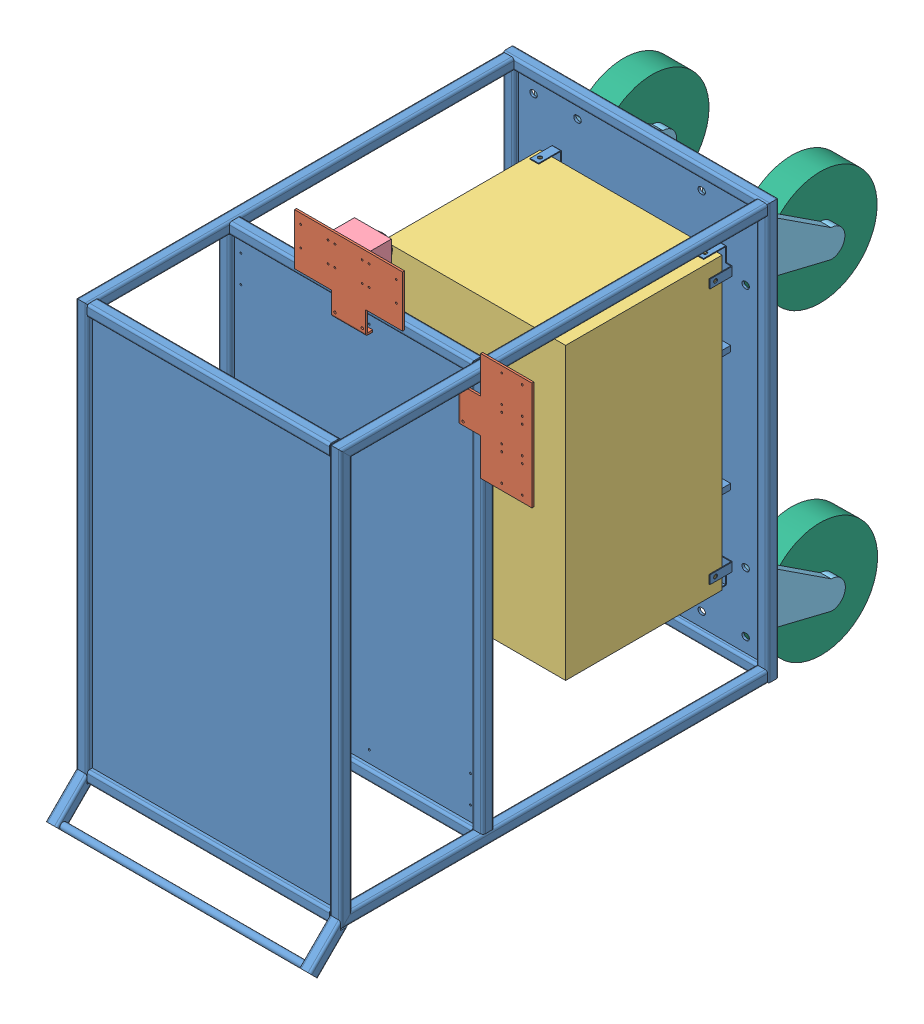
SolidWorks assembly kart, configuration Default. Lengths in mm.
Overall size (555.49 886.14 1699.31).
17 component instances, 6 part files, 21 mates.
Components (placement in the parent):
- kart_skeleton-1: kart_skeleton [Default<A macchina>] at (18.5226 -16.0189 875.6692) size (465.49 783.64 823.64)
- lidar_plate_T-1: lidar_plate_T [Default] at (296.2677 278.9811 1389.6647) x (-1 0 0) z (0 0 1) size (130.26 190 13)
- lidar_plate_T-2: lidar_plate_T [Default] at (18.5226 383.9811 1389.1692) x (0 -1 0) z (0 0 1) size (130.26 190 13)
- battery_mockup-1: battery_mockup [Default] at (18.5226 -16.0189 1030.1692) x (0 1 0) z (1 0 0) size (510 275 320)
- lidar-1: lidar [Default] at (18.5226 393.9811 1346.1692) size (72 65 60)
- castor-1: castor [Default] at (-42.7723 235.0131 796.9372) x (0 1 0) z (1 0 0) size (209 240.65 88)
  - pivot-1: pivot [Default] at (16.468 69.732 165.04) size (133.39 165.04 88)
  - wheel-1: wheel [Default] at (-42.532 -63.918 209.04) size (200 200 50)
- castor-2: castor [Default] at (-338.2625 235.0131 796.9372) x (0 1 0) z (1 0 0) size (209 240.65 88)
  - pivot-1: pivot [Default] at (16.468 69.732 165.04) size (133.39 165.04 88)
  - wheel-1: wheel [Default] at (-42.532 -63.918 209.04) size (200 200 50)
- castor-3: castor [Default] at (-42.5347 -302.7664 796.9372) x (-0.013303 0.999912 0) z (0.999912 0.013303 0) size (209 240.65 88)
  - pivot-1: pivot [Default] at (16.468 69.732 165.04) size (133.39 165.04 88)
  - wheel-1: wheel [Default] at (-42.532 -63.918 209.04) size (200 200 50)
- castor-4: castor [Default] at (-338.3665 -298.6093 796.9372) x (0.006589 0.999978 0) z (0.999978 -0.006589 0) size (209 240.65 88)
  - pivot-1: pivot [Default] at (16.468 69.732 165.04) size (133.39 165.04 88)
  - wheel-1: wheel [Default] at (-42.532 -63.918 209.04) size (200 200 50)
Mates (geometry in assembly coordinates):
- Parallelo1: parallel aligned: plane of kart_skeleton-1 through (247.2677 328.9811 875.6692) normal (0 -1 0); plane of lidar_plate_T-1 through (341.2677 183.9811 1386.1647) normal (0 -1 0)
- Coincidente19: coincident anti-aligned: plane of kart_skeleton-1 through (251.2677 332.9811 875.6692) normal (1 0 0); plane of lidar_plate_T-1 through (251.2677 308.9811 1386.1647) normal (-1 0 0)
- Concentrico20: concentric aligned: cylinder of kart_skeleton-1 through (220.2677 254.9811 1376.6692) axis (0 0 1) radius 1.65; cylinder of lidar_plate_T-1 through (220.2677 254.9811 1389.6647) axis (0 0 1) radius 2.15
- Concentrico21: concentric aligned: cylinder of kart_skeleton-1 through (220.2677 302.9811 1376.6692) axis (0 0 1) radius 1.65; cylinder of lidar_plate_T-1 through (220.2677 302.9811 1389.6647) axis (0 0 1) radius 2.15
- Coincidente25: coincident anti-aligned: plane of kart_skeleton-1 through (231.2677 348.9831 1376.6692) normal (0 0 1); plane of lidar_plate_T-1 through (214.5121 248.9811 1376.6692) normal (0 0 -1)
- Coincidente26: coincident anti-aligned: plane of kart_skeleton-1 through (-204.2225 344.9811 1385.6692) normal (0 0 1); plane of lidar_plate_T-2 through (18.5226 383.9811 1385.6692) normal (0 0 -1)
- Concentrico26: concentric aligned: cylinder of lidar_plate_T-2 through (42.5226 307.9811 1389.1692) axis (0 0 1) radius 2.15; cylinder of kart_skeleton-1 through (42.5226 307.9811 1376.6692) axis (0 0 1) radius 1.65
- Concentrico27: concentric aligned: cylinder of kart_skeleton-1 through (-5.4774 307.9811 1376.6692) axis (0 0 1) radius 1.65; cylinder of lidar_plate_T-2 through (-5.4774 307.9811 1389.1692) axis (0 0 1) radius 2.15
- Concentrico37: concentric aligned: cylinder of kart_skeleton-1 through (182.0226 208.9811 907.6692) axis (1 0 0) radius 3.4; cylinder of battery_mockup-1 through (178.5226 208.9811 907.6692) axis (1 0 0) radius 3.4
- Concentrico39: concentric aligned: cylinder of kart_skeleton-1 through (163.5226 242.4811 907.6692) axis (0 1 0) radius 3.4; cylinder of battery_mockup-1 through (163.5226 238.9811 907.6692) axis (0 1 0) radius 3.4
- Concentrico40: concentric aligned: cylinder of lidar_plate_T-2 through (42.5226 411.9811 1389.1692) axis (0 0 1) radius 1.6; cylinder of lidar-1 through (42.5226 411.9811 1385.6692) axis (0 0 1) radius 1.25
- Concentrico41: concentric aligned: cylinder of lidar_plate_T-2 through (42.5226 375.9811 1389.1692) axis (0 0 1) radius 1.6; cylinder of lidar-1 through (42.5226 375.9811 1385.6692) axis (0 0 1) radius 1.25
- Coincidente30: coincident anti-aligned: plane of lidar_plate_T-2 through (18.5226 383.9811 1385.6692) normal (0 0 -1); plane of lidar-1 through (18.5226 393.9811 1385.6692) normal (0 0 1)
- Coincidente31: coincident anti-aligned: plane of kart_skeleton-1 through (231.2677 348.9831 873.6692) normal (0 0 -1); plane of castor-1/pivot-1 through (166.2677 251.4811 873.6692) normal (0 0 1)
- Coincidente32: coincident: point of kart_skeleton-1; point of castor-1/pivot-1
- Coincidente33: coincident anti-aligned: plane of kart_skeleton-1 through (231.2677 348.9831 873.6692) normal (0 0 -1); plane of castor-2/pivot-1 through (-129.2225 251.4811 873.6692) normal (0 0 1)
- Coincidente35: coincident: point of kart_skeleton-1; point of castor-2/pivot-1
- Coincidente36: coincident: point of kart_skeleton-1; point of castor-3/pivot-1
- Coincidente37: coincident anti-aligned: plane of kart_skeleton-1 through (231.2677 348.9831 873.6692) normal (0 0 -1); plane of castor-3/pivot-1 through (166.2677 -283.5189 873.6692) normal (0 0 1)
- Coincidente38: coincident: point of kart_skeleton-1; point of castor-4/pivot-1
- Coincidente39: coincident anti-aligned: plane of kart_skeleton-1 through (231.2677 348.9831 873.6692) normal (0 0 -1); plane of castor-4/pivot-1 through (-129.2225 -283.5189 873.6692) normal (0 0 1)
